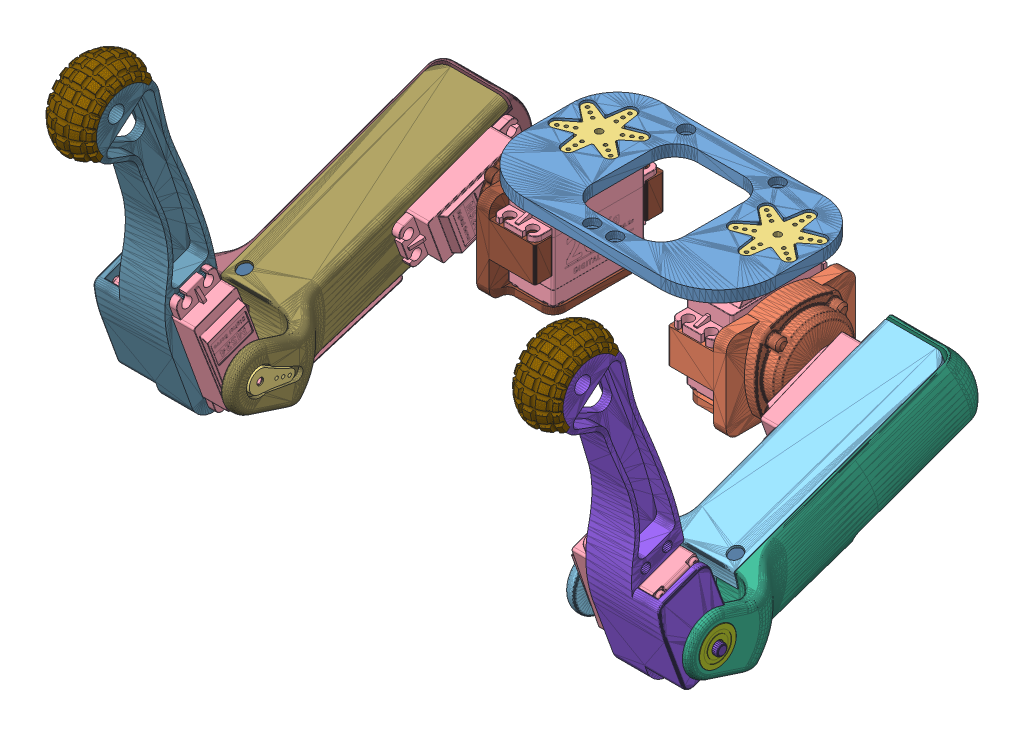
SolidWorks assembly Front Legs, configuration Default. Lengths in mm.
Overall size (257.32 168.18 205.82).
53 component instances, 14 part files, 6 mates.
Components (placement in the parent):
- 7_Rear_shoulder-2: 7_Rear_shoulder [Default] at (-12.5249 87.612 92.1876) size (110 5 66)
- Left Leg Assembly-1: Left Leg Assembly [Default] at (86.5165 30.9423 148.2853) size (111.25 167.25 201.66)
  - Left_arm_joint_mg-1: Left_arm_joint_mg [Default] at (-15.0415 19.5698 -40.5977) size (37.5 46 56.5)
  - Servohorn-1: Servohorn [4 Prong] at (19.6585 29.8198 -20.3477) x (0 -0.592234 0.805766) z (-1 0 0) size (31.8 31.8 2.24)
  - Servo Motor-1: Servo Motor [Default] at (-5.0415 40.5698 -30.0977) size (20.1 45.99 55.6)
  - Servohorn-2: Servohorn [Default] at (-5.0415 60.9698 -30.0977) x (0.506689 0 -0.862129) z (0 -1 0) size (28.18 31.8 2.24)
  - Servo Motor-2: Servo Motor [Default] at (38.0585 29.8198 -20.3477) x (0 0.939693 0.34202) z (0 -0.34202 0.939693) size (20.1 45.99 55.6)
  - Left_arm_mg-1: Left_arm_mg [Default] at (38.0585 42.7737 -26.7003) x (0 -0.939693 -0.34202) z (0 -0.34202 0.939693) size (38.24 39.8 137.4)
  - SM_Left_arm_cover-1: SM_Left_arm_cover [Default] at (38.2585 50.3364 -32.5645) x (0 -0.939693 -0.34202) z (0 -0.34202 0.939693) size (41.16 45 143.55)
  - F625ZZ Ball Bearing-1: F625ZZ Ball Bearing [Default] at (78.2585 -1.6568 83.7617) x (0 -0.070361 0.997522) z (-1 0 0) size (18 18 5)
  - Servohorn-3: Servohorn [1 Prong] at (28.0585 6.3719 84.4796) x (0 0.893193 -0.449674) z (1 0 0) size (9.55 20.65 2.24)
  - Left_wrist_mg-1: Left_wrist_mg [Default] at (18.4585 0.3781 71.7095) x (0 0.939693 0.34202) z (0 -0.34202 0.939693) size (149.99 36.9 30)
  - foot-1: foot [Default] at (48.4585 115.3593 124.2008) x (0 0.642788 -0.766044) z (0 -0.766044 -0.642788) size (38.32 20 19.41)
  - Servo Motor-3: Servo Motor [Default] at (48.4585 6.3719 84.4796) x (0 0.34202 -0.939693) z (0 0.939693 0.34202) size (20.1 45.99 55.6)
  - _Hex_Screws-1: _Hex_Screws [H M4x20] at (-0.0415 43.7698 3.9023) x (-0.837169 0 -0.546944) z (-0.546944 0 0.837169) size (7 22.8 8.08) (hidden)
  - _Hex_Screws-2: _Hex_Screws [H M4x20] at (-10.0415 43.7698 -44.0977) x (-0.837169 0 -0.546944) z (-0.546944 0 0.837169) size (7 22.8 8.08) (hidden)
  - _Hex_Screws-3: _Hex_Screws [H M4x20] at (-10.0415 43.7698 3.9023) x (-0.837169 0 -0.546944) z (-0.546944 0 0.837169) size (7 22.8 8.08) (hidden)
  - _Hex_Screws-4: _Hex_Screws [H M4x20] at (-0.0415 43.7698 -44.0977) x (-0.837169 0 -0.546944) z (-0.546944 0 0.837169) size (7 22.8 8.08) (hidden)
  - _Hex_Screws-5: _Hex_Screws [H M4x20] at (34.8585 22.8895 13.3119) x (0 0.825172 -0.564882) z (0 -0.564882 -0.825172) size (7 22.8 8.08) (hidden)
  - _Hex_Screws-6: _Hex_Screws [H M4x20] at (34.8585 13.4926 9.8917) x (0 0.825172 -0.564882) z (0 -0.564882 -0.825172) size (7 22.8 8.08) (hidden)
  - _Hex_Screws-7: _Hex_Screws [H M4x20] at (34.8585 39.3065 -31.7933) x (0 0.802845 -0.596188) z (0 -0.596188 -0.802845) size (7 22.8 8.08) (hidden)
  - _Hex_Screws-8: _Hex_Screws [H M4x20] at (34.8585 29.9096 -35.2135) x (0 -0.944714 0.327896) z (0 0.327896 0.944714) size (7 22.8 8.08) (hidden)
  - _Hex_Screws-9: _Hex_Screws [H M4x20] at (45.2585 40.0315 91.4099) x (0 0.825172 -0.564882) z (0 -0.564882 -0.825172) size (7 22.8 8.08) (hidden)
  - _Hex_Screws-10: _Hex_Screws [H M4x20] at (45.2585 36.6113 100.8068) x (0 0.825172 -0.564882) z (0 -0.564882 -0.825172) size (7 22.8 8.08) (hidden)
  - _Hex_Screws-11: _Hex_Screws [H M4x20] at (45.2585 -5.0737 74.9929) x (0 0.825172 -0.564882) z (0 -0.564882 -0.825172) size (7 22.8 8.08) (hidden)
  - _Hex_Screws-12: _Hex_Screws [H M4x20] at (45.2585 -8.4939 84.3898) x (0 0.825172 -0.564882) z (0 -0.564882 -0.825172) size (7 22.8 8.08) (hidden)
  - _Hex_Screws-13: _Hex_Screws [H M3x16] at (62.9617 14.9879 55.4881) x (0.992954 0.04053 -0.111356) z (-0.118503 0.33961 -0.933071) size (5.5 18 6.35)
- Right Leg Assembly-1: Right Leg Assembly [Default] at (19.1728 32.9715 132.7261) size (64.22 167.45 199.81)
  - Right_arm_joint_mg-1: Right_arm_joint_mg [Default] at (24.2858 18.5405 -25.0321) size (37.5 46 56.5)
  - Servohorn-1: Servohorn [4 Prong] at (-38.4142 28.7905 -4.7821) x (0 0.715501 0.698611) z (-1 0 0) size (31.8 31.8 2.24)
  - Servo Motor-1: Servo Motor [Default] at (-15.7142 38.5405 -14.5321) size (20.1 45.99 55.6)
  - Servohorn-2: Servohorn [Default] at (-15.7142 58.9405 -14.5321) x (-0.99999 0 0.00451) z (0 -1 0) size (28.18 31.8 2.24)
  - Right_arm_mg-1: Right_arm_mg [Default] at (-8.8142 41.6076 -10.7588) x (0 -0.939693 -0.34202) z (0 -0.34202 0.939693) size (38.24 39.8 137.4)
  - SM_Right_arm_cover-1: SM_Right_arm_cover [Default] at (-48.6142 49.0427 -16.5661) x (0 -0.939693 -0.34202) z (0 -0.34202 0.939693) size (41.16 45 143.55)
  - F625ZZ Ball Bearing-1: F625ZZ Ball Bearing [Default] at (-98.6142 -2.6723 100.0196) x (0 0.0383 -0.999266) z (1 0 0) size (18 18 5)
  - Servohorn-3: Servohorn [1 Prong] at (-48.8142 5.2058 100.4211) x (0 -0.953491 0.301422) z (-1 0 0) size (9.55 20.65 2.24)
  - Servo Motor-2: Servo Motor [Default] at (-67.7142 5.2058 100.4211) x (0 -0.34202 0.939693) z (0 0.939693 0.34202) size (20.1 45.99 55.6)
  - Servo Motor-3: Servo Motor [Default] at (-58.8142 28.7905 -4.7821) x (0 -0.939693 -0.34202) z (0 -0.34202 0.939693) size (20.1 45.99 55.6)
  - Right_wrist_mg-1: Right_wrist_mg [Default] at (-67.7142 -0.7709 87.604) x (0 0.939693 0.34202) z (0 -0.34202 0.939693) size (149.99 36.9 30)
  - foot-1: foot [Default] at (-67.7142 114.2242 140.0873) x (0 -0.656061 0.754708) z (0 -0.754708 -0.656061) size (38.32 20 19.41)
  - _Hex_Screws-1: _Hex_Screws [H M4x20] at (-20.7142 41.7405 19.4679) x (-0.837169 0 -0.546944) z (-0.546944 0 0.837169) size (7 22.8 8.08) (hidden)
  - _Hex_Screws-2: _Hex_Screws [H M4x20] at (-10.7142 41.7405 -28.5321) x (-0.837169 0 -0.546944) z (-0.546944 0 0.837169) size (7 22.8 8.08) (hidden)
  - _Hex_Screws-3: _Hex_Screws [H M4x20] at (-10.7142 41.7405 19.4679) x (-0.99108 0 -0.133267) z (-0.133267 0 0.99108) size (7 22.8 8.08) (hidden)
  - _Hex_Screws-4: _Hex_Screws [H M4x20] at (-20.7142 41.7405 -28.5321) x (0.837169 0 0.546944) z (0.546944 0 -0.837169) size (7 22.8 8.08) (hidden)
  - _Hex_Screws-5: _Hex_Screws [H M4x20] at (-55.6142 28.8803 -19.6479) x (0 0.085299 -0.996355) z (0 0.996355 0.085299) size (7 22.8 8.08) (hidden)
  - _Hex_Screws-8: _Hex_Screws [H M4x20] at (-55.6142 12.4633 25.4573) x (0 -0.381849 0.924225) z (0 -0.924225 -0.381849) size (7 22.8 8.08) (hidden)
  - _Hex_Screws-9: _Hex_Screws [H M4x20] at (-55.6142 21.8603 28.8775) x (0 -0.381849 0.924225) z (0 -0.924225 -0.381849) size (7 22.8 8.08) (hidden)
  - _Hex_Screws-10: _Hex_Screws [H M4x20] at (-64.5142 -9.66 100.3313) x (0 -0.381849 0.924225) z (0 -0.924225 -0.381849) size (7 22.8 8.08) (hidden)
  - _Hex_Screws-11: _Hex_Screws [H M4x20] at (-64.5142 38.8655 107.3514) x (0 -0.381849 0.924225) z (0 -0.924225 -0.381849) size (7 22.8 8.08) (hidden)
  - _Hex_Screws-12: _Hex_Screws [H M4x20] at (-64.5142 -6.2398 90.9344) x (0 -0.381849 0.924225) z (0 -0.924225 -0.381849) size (7 22.8 8.08) (hidden)
  - _Hex_Screws-14: _Hex_Screws [H M4x20] at (-64.5142 35.4453 116.7483) x (0 -0.381849 0.924225) z (0 -0.924225 -0.381849) size (7 22.8 8.08) (hidden)
  - _Hex_Screws-15: _Hex_Screws [H M4x20] at (-55.6142 38.2772 -16.2277) x (0 0.381849 -0.924225) z (0 0.924225 0.381849) size (7 22.8 8.08) (hidden)
  - _Hex_Screws-19: _Hex_Screws [H M3x16] at (-83.8911 13.8209 71.432) x (0.19625 0.335369 -0.921419) z (-0.980554 0.067122 -0.184415) size (5.5 18 6.35)
Mates (geometry in assembly coordinates):
- Distance1: distance = 2 mm aligned: plane of 7_Rear_shoulder-2 through (-12.5249 89.912 92.1876) normal (0 1 0); plane of Left Leg Assembly-1/Servohorn-2 through (81.4751 91.912 118.1876) normal (0 1 0)
- Parallel1: parallel aligned: plane of 7_Rear_shoulder-2 through (-12.5249 87.612 94.1876) normal (0 0 -1); plane of Left Leg Assembly-1/Left_arm_joint_mg-1 through (71.4751 50.512 99.6876) normal (0 0 -1)
- Distance2: distance = 2 mm aligned: plane of 7_Rear_shoulder-2 through (-12.5249 89.912 92.1876) normal (0 1 0); plane of Right Leg Assembly-1/Servohorn-2 through (3.4586 91.912 118.194) normal (0 1 0)
- Parallel2: parallel aligned: plane of 7_Rear_shoulder-2 through (-12.5249 87.612 94.1876) normal (0 0 -1); plane of Right Leg Assembly-1/Right_arm_joint_mg-1 through (43.4586 51.512 99.694) normal (0 0 -1)
- Coincident1: coincident: point of 7_Rear_shoulder-2; line of Right Leg Assembly-1/Servohorn-2 through (3.4586 91.912 118.194) axis (0 1 0)
- Coincident2: coincident: point of 7_Rear_shoulder-2; line of Left Leg Assembly-1/Servohorn-2 through (81.4751 91.912 118.1876) axis (0 1 0)
